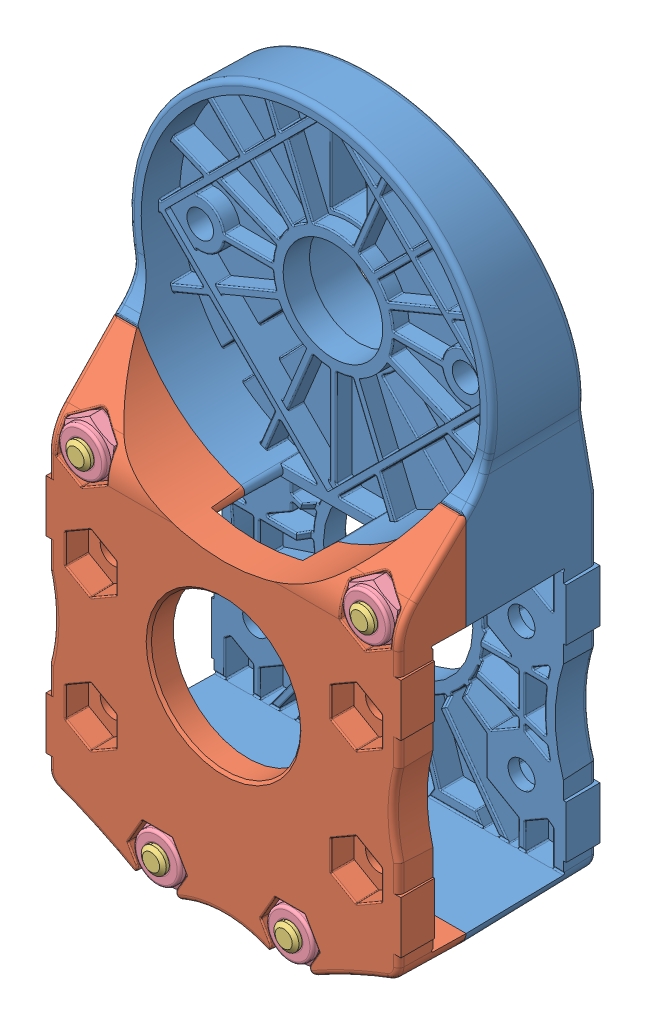
SolidWorks assembly 217-4156-STEP-20140806, configuration Default. Lengths in mm.
Overall size (69.6 130.19 39.75).
10 component instances, 4 part files, 0 mates.
Components (placement in the parent):
- 217-4156-001 Rev6-1: 217-4156-001 Rev6 [Default] at origin size (69.6 129.7 26.08)
- 217-4156-002 Rev5-1: 217-4156-002 Rev5 [Default] at origin size (67.92 80.13 15.71)
- 217-4155-003 Rev1_SSA1032-1375ZB-1: 217-4155-003 Rev1_SSA1032-1375ZB [Default] at (-27.15 30.0962 -21.05) x (0.999179 -0.040505 0) z (0.040505 0.999179 0) size (7.87 39.75 7.87)
- 217-4155-003 Rev1_SSA1032-1375ZB-2: 217-4155-003 Rev1_SSA1032-1375ZB [Default] at (27.15 30.0962 -21.05) x (1 0 0) z (0 1 0) size (7.87 39.75 7.87)
- 217-4155-003 Rev1_SSA1032-1375ZB-3: 217-4155-003 Rev1_SSA1032-1375ZB [Default] at (12.7 -29.8538 -21.05) x (1 0 0) z (0 1 0) size (7.87 39.75 7.87)
- 217-4155-003 Rev1_SSA1032-1375ZB-4: 217-4155-003 Rev1_SSA1032-1375ZB [Default] at (-12.7 -29.8538 -21.05) x (1 0 0) z (0 1 0) size (7.87 39.75 7.87)
- 217-4155-002 Rev2_NNY1032-ZC-1: 217-4155-002 Rev2_NNY1032-ZC [Default] at (-27.15 30.0962 8.35) x (-0.5 0.866025 0) z (0 0 1) size (9.39 10.84 4.45)
- 217-4155-002 Rev2_NNY1032-ZC-2: 217-4155-002 Rev2_NNY1032-ZC [Default] at (27.15 30.0962 8.35) size (9.39 10.84 4.45)
- 217-4155-002 Rev2_NNY1032-ZC-3: 217-4155-002 Rev2_NNY1032-ZC [Default] at (-12.7 -29.8538 8.35) x (0.866025 -0.5 0) z (0 0 1) size (9.39 10.84 4.45)
- 217-4155-002 Rev2_NNY1032-ZC-4: 217-4155-002 Rev2_NNY1032-ZC [Default] at (12.7 -29.8538 8.35) x (0.866025 -0.5 0) z (0 0 1) size (9.39 10.84 4.45)
